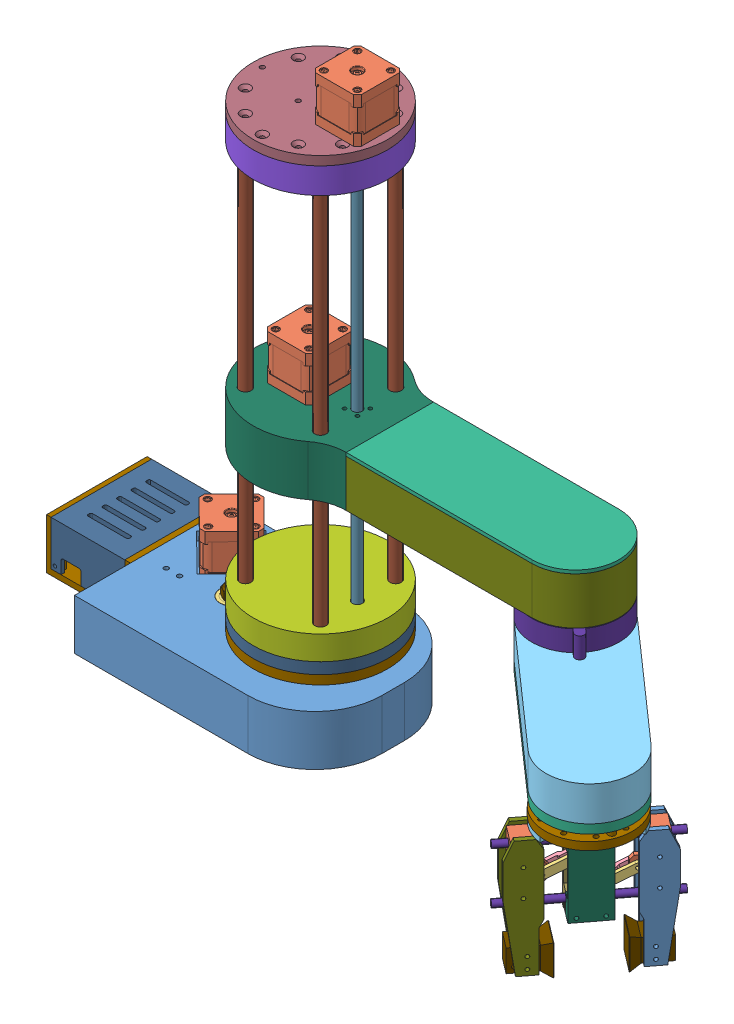
SolidWorks assembly SCARA Robot, configuration SCARA Robot. Lengths in mm. (continued)
Mates (geometry in assembly coordinates): (continued)
- Concentric43: concentric aligned: cylinder of Smooth Rod D10mm L400mm-2 through (76.0876 425 33.5876) axis (0 -1 0) radius 5; cylinder of Z-axis Mount Platform-1 through (76.0876 211.1984 33.5876) axis (0 -1 0) radius 5.25
- Concentric44: concentric anti-aligned: cylinder of Z-axis Mount Platform-1 through (-17.501 182.6984 -25.5) axis (1 0 0) radius 2.55; cylinder of Arm 1-1 through (309.501 182.6984 -25.5) axis (-1 0 0) radius 2.55
- Coincident31: coincident anti-aligned: plane of Z-axis Mount Platform-1 through (104.5 166.1984 0) normal (1 0 0); plane of Arm 1-1 through (104.5 176.1984 -39) normal (-1 0 0)
- Concentric451: concentric aligned: cylinder of Arm 1-1 through (180.5 182.1984 0) axis (0 -1 0) radius 11; cylinder of Ball Bearing 608 - 8x22x7mm-5 through (180.5 175.3984 0) axis (0 -1 0) radius 8.25
- Coincident321: coincident anti-aligned: plane of Arm 1-1 through (180.5 175.1984 0) normal (0 1 0); plane of Ball Bearing 608 - 8x22x7mm-5 through (180.5 175.1984 0) normal (0 -1 0)
- Coincident33: coincident anti-aligned: plane of Arm 1-1 through (180.5 173.1984 0) normal (0 -1 0); plane of Ball Bearing 608 - 8x22x7mm-6 through (180.5 173.1984 0) normal (0 1 0)
- Concentric46: concentric anti-aligned: cylinder of Arm 1-1 through (180.5 173.1984 0) axis (0 -1 0) radius 11; cylinder of Ball Bearing 608 - 8x22x7mm-6 through (180.5 166.1984 0) axis (0 1 0) radius 11
- Coincident34: coincident anti-aligned: plane of J2 Coupler-1 through (270.5 154.1984 0) normal (0 1 0); plane of Thrust Bearing 35x52x12mm-1 through (270.5 154.1984 0) normal (0 -1 0)
- Concentric47: concentric anti-aligned: cylinder of J2 Coupler-1 through (270.5 154.1984 0) axis (0 1 0) radius 26.5; cylinder of Thrust Bearing 35x52x12mm-1 through (270.5 166.1984 0) axis (0 -1 0) radius 26
- Concentric48: concentric anti-aligned: cylinder of Arm 1-1 through (270.5 169.1984 0) axis (0 1 0) radius 21; cylinder of Ball Bearing 30x42x7mm-1 through (270.5 176.1984 0) axis (0 -1 0) radius 21
- Coincident35: coincident anti-aligned: plane of Arm 1-1 through (270.5 169.1984 0) normal (0 1 0); plane of Ball Bearing 30x42x7mm-1 through (270.5 169.1984 0) normal (0 -1 0)
- Concentric49: concentric anti-aligned: cylinder of Arm 1-1 through (270.5 166.1984 0) axis (0 1 0) radius 17.5; cylinder of J2 Coupler-1 through (270.5 171.1984 0) axis (0 -1 0) radius 15
- Coincident36: coincident anti-aligned: plane of Arm 1-1 through (270.5 166.1984 0) normal (0 -1 0); plane of Thrust Bearing 35x52x12mm-1 through (270.5 166.1984 0) normal (0 1 0)
- Concentric50: concentric anti-aligned: cylinder of Ball Bearing 608 - 8x22x7mm-5 through (180.5 175.1984 0) axis (0 1 0) radius 4; cylinder of GT2 Pulley - 23 - 80 teeth-1 through (180.5 202.1984 0) axis (0 -1 0) radius 4
- Concentric51: concentric aligned: cylinder of J2 Coupler-1 through (270.5 147.1984 0) axis (0 1 0) radius 6.25; cylinder of GT2 Pulley - 92 teeth - J2-1 through (270.5 172.1984 0) axis (0 1 0) radius 6.25
- Coincident38: coincident anti-aligned: plane of GT2 Pulley - 92 teeth - J2-1 through (270.5 188.1984 0) normal (0 -1 0); plane of Thrust Bearing 35x52x12mm-2 through (270.5 188.1984 0) normal (0 1 0)
- Concentric52: concentric anti-aligned: cylinder of GT2 Pulley - 92 teeth - J2-1 through (270.5 172.1984 0) axis (0 1 0) radius 15; cylinder of Thrust Bearing 35x52x12mm-2 through (270.5 179.9984 0) axis (0 -1 0) radius 17.5
- Coincident39: coincident anti-aligned: plane of Arm 1-1 through (270.5 176.1984 0) normal (0 1 0); plane of Thrust Bearing 35x52x12mm-2 through (270.5 176.1984 0) normal (0 -1 0)
- Concentric53: concentric anti-aligned: cylinder of Z-axis Mount Platform-1 through (-17.501 200.6984 -25.5) axis (1 0 0) radius 2.55; cylinder of Arm 1-1 through (309.501 200.6984 -25.5) axis (-1 0 0) radius 2.55
- Concentric54: concentric aligned: cylinder of Z-axis Mount Platform-1 through (32.5 166.1984 0) axis (0 1 0) radius 12.5; cylinder of Stepper NEMA 17 -  20mm shaft-3 through (32.5 189.1984 0) axis (0 1 0) radius 2.5
- Concentric55: concentric anti-aligned: cylinder of Z-axis Mount Platform-1 through (17 166.1984 15.5) axis (0 1 0) radius 1.6; cylinder of Stepper NEMA 17 -  20mm shaft-3 through (17 215.1984 15.5) axis (0 -1 0) radius 1.5
- Coincident40: coincident anti-aligned: plane of Z-axis Mount Platform-1 through (42.5 211.1984 0) normal (0 1 0); plane of Stepper NEMA 17 -  20mm shaft-3 through (12 211.1984 0) normal (0 -1 0)
- Concentric56: concentric anti-aligned: cylinder of Stepper NEMA 17 -  20mm shaft-3 through (32.5 189.1984 0) axis (0 1 0) radius 2.5; cylinder of GT2 Pulley - Parametric-2 through (32.5 207.9984 0) axis (0 -1 0) radius 7.3122
- Coincident41: coincident aligned: plane of GT2 Pulley - 23 - 80 teeth-1 through (180.5 193.9984 0) normal (0 1 0); plane of GT2 Pulley - Parametric-2 through (32.5 193.9984 0) normal (0 1 0)
- Coincident42: coincident anti-aligned: plane of GT2 Pulley - 23 - 80 teeth-1 through (180.5 183.3984 0) normal (0 -1 0); plane of M8 Washer-3 through (180.5 183.3984 0) normal (0 1 0)
- Concentric57: concentric aligned: cylinder of GT2 Pulley - 23 - 80 teeth-1 through (180.5 202.1984 0) axis (0 -1 0) radius 4; cylinder of M8 Washer-3 through (180.5 183.3984 0) axis (0 -1 0) radius 7
- Coincident43: coincident anti-aligned: plane of Ball Bearing 608 - 8x22x7mm-5 through (180.5 182.1984 0) normal (0 1 0); plane of M8 Washer-3 through (180.5 182.1984 0) normal (0 -1 0)
- Concentric58: concentric anti-aligned: cylinder of Z-axis Mount Platform-1 through (8.9124 166.1984 33.5876) axis (0 1 0) radius 9.5; cylinder of Linear Bearing 10x19x29mm-3 through (8.9124 205.1984 33.5876) axis (0 -1 0) radius 9.5
- Coincident44: coincident anti-aligned: plane of Z-axis Mount Platform-1 through (104.4919 205.1984 81) normal (0 -1 0); plane of Linear Bearing 10x19x29mm-3 through (8.9124 205.1984 33.5876) normal (0 1 0)
- Coincident45: coincident anti-aligned: plane of Z-axis Mount Platform-1 through (104.4919 205.1984 81) normal (0 -1 0); plane of Linear Bearing 10x19x29mm-6 through (76.0876 205.1984 33.5876) normal (0 1 0)
- Concentric59: concentric anti-aligned: cylinder of Z-axis Mount Platform-1 through (76.0876 166.1984 33.5876) axis (0 1 0) radius 9.5; cylinder of Linear Bearing 10x19x29mm-6 through (76.0876 205.1984 33.5876) axis (0 -1 0) radius 5
- Concentric60: concentric anti-aligned: cylinder of Z-axis Mount Platform-1 through (76.0876 166.1984 -33.5876) axis (0 1 0) radius 9.5; cylinder of Linear Bearing 10x19x29mm-2 through (76.0876 205.1984 -33.5876) axis (0 -1 0) radius 9.5
- Coincident46: coincident anti-aligned: plane of Z-axis Mount Platform-1 through (104.4919 205.1984 81) normal (0 -1 0); plane of Linear Bearing 10x19x29mm-2 through (76.0876 205.1984 -33.5876) normal (0 1 0)
- Concentric61: concentric anti-aligned: cylinder of Z-axis Mount Platform-1 through (8.9124 166.1984 -33.5876) axis (0 1 0) radius 9.5; cylinder of Linear Bearing 10x19x29mm-1 through (8.9124 205.1984 -33.5876) axis (0 -1 0) radius 9.5
- Coincident47: coincident anti-aligned: plane of Z-axis Mount Platform-1 through (104.4919 205.1984 81) normal (0 -1 0); plane of Linear Bearing 10x19x29mm-1 through (8.9124 205.1984 -33.5876) normal (0 1 0)
- Parallel3: parallel aligned: plane of Base-1 through (-107.5 10 70) normal (0 0 1); plane of Arm 1-1 through (104.5 176.1984 39) normal (0 0 1)
- Concentric62: concentric aligned: cylinder of J2 Coupler-1 through (270.5 165.6984 0) axis (0 -1 0) radius 39; cylinder of Arm 2-1 through (270.5 147.1984 0) axis (0 -1 0) radius 17
- Coincident49: coincident anti-aligned: plane of J2 Coupler-1 through (270.5 147.1984 0) normal (0 -1 0); plane of Arm 2-1 through (270.5 147.1984 0) normal (0 1 0)
- Concentric63: concentric anti-aligned: cylinder of J2 Coupler-1 through (280.4501 147.1984 29.6236) axis (0 1 0) radius 2.05; cylinder of Arm 2-1 through (280.4501 147.1984 29.6236) axis (0 -1 0) radius 2.05
- Concentric64: concentric anti-aligned: cylinder of Arm 2-1 through (270.5 141.1984 0) axis (0 1 0) radius 39; cylinder of Arm 2 Cover-1 through (270.5 116.1984 0) axis (0 -1 0) radius 39
- Coincident50: coincident anti-aligned: plane of Arm 2-1 through (270.5 116.1984 0) normal (0 -1 0); plane of Arm 2 Cover-1 through (270.5 116.1984 0) normal (0 1 0)
- Concentric65: concentric anti-aligned: cylinder of Arm 2-1 through (378.46 141.1984 95.2924) axis (0 1 0) radius 39; cylinder of Arm 2 Cover-1 through (378.46 116.1984 95.2924) axis (0 -1 0) radius 39
- Concentric66: concentric anti-aligned: cylinder of Arm 1-1 through (220.888 166.1984 5) axis (0 1 0) radius 1.6; cylinder of Micro switch-1 through (220.888 166.1984 5) axis (0 -1 0) radius 1.5
- Concentric67: concentric anti-aligned: cylinder of Arm 1-1 through (212.5 166.1984 9.46) axis (0 1 0) radius 1.6; cylinder of Micro switch-1 through (212.5 166.1984 9.46) axis (0 -1 0) radius 1.5
- Coincident51: coincident anti-aligned: plane of Arm 1-1 through (270.5 166.1984 0) normal (0 -1 0); plane of Micro switch-1 through (217.6469 166.1984 9.5547) normal (0 1 0)
- Concentric68: concentric anti-aligned: cylinder of Arm 2 Cover-1 through (266.0017 108.1984 -3.9705) axis (0 1 0) radius 12.5; cylinder of NEMA 17 Stepper L24mm - 20mm shaft-1 through (266.0017 130.1984 -3.9705) axis (0 -1 0) radius 2.5
- Concentric69: concentric aligned: cylinder of Arm 2 Cover-1 through (267.3652 108.1984 17.9073) axis (0 1 0) radius 1.6; cylinder of NEMA 17 Stepper L24mm - 20mm shaft-1 through (267.3652 103.8984 17.9073) axis (0 1 0) radius 1.5
- Coincident52: coincident anti-aligned: plane of Arm 2 Cover-1 through (270.5 108.1984 0) normal (0 -1 0); plane of NEMA 17 Stepper L24mm - 20mm shaft-1 through (266.0017 108.1984 -3.9705) normal (0 1 0)
- Concentric701: concentric aligned: cylinder of Arm 2 Cover-1 through (372.8371 109.1984 90.3293) axis (0 1 0) radius 21; cylinder of Ball Bearing 30x42x7mm-2 through (372.8371 109.1984 90.3293) axis (0 1 0) radius 21
- Coincident53: coincident anti-aligned: plane of Arm 2 Cover-1 through (372.8371 109.1984 90.3293) normal (0 1 0); plane of Ball Bearing 30x42x7mm-2 through (372.8371 109.1984 90.3293) normal (0 -1 0)
- Concentric71: concentric anti-aligned: cylinder of Ball Bearing 30x42x7mm-2 through (372.8371 109.1984 90.3293) axis (0 1 0) radius 15; cylinder of Thrust Bearing 35x52x12mm-3 through (372.8371 119.9984 90.3293) axis (0 -1 0) radius 17.5
- Coincident54: coincident anti-aligned: plane of Arm 2 Cover-1 through (270.5 116.1984 0) normal (0 1 0); plane of Thrust Bearing 35x52x12mm-3 through (372.8371 116.1984 90.3293) normal (0 -1 0)
- Concentric73: concentric aligned: cylinder of Ball Bearing 30x42x7mm-2 through (372.8371 109.1984 90.3293) axis (0 1 0) radius 15; cylinder of Thrust Bearing 35x52x12mm-4 through (372.8371 96.1984 90.3293) axis (0 1 0) radius 17.5
- Coincident55: coincident anti-aligned: plane of Arm 2 Cover-1 through (270.5 108.1984 0) normal (0 -1 0); plane of Thrust Bearing 35x52x12mm-4 through (372.8371 108.1984 90.3293) normal (0 1 0)
- Concentric74: concentric anti-aligned: cylinder of J3 Coupler-1 through (372.8371 107.6984 90.3293) axis (0 -1 0) radius 26.5; cylinder of Thrust Bearing 35x52x12mm-4 through (372.8371 96.1984 90.3293) axis (0 1 0) radius 26
- Coincident56: coincident anti-aligned: plane of J3 Coupler-1 through (372.8371 96.1984 90.3293) normal (0 1 0); plane of Thrust Bearing 35x52x12mm-4 through (372.8371 96.1984 90.3293) normal (0 -1 0)
- Concentric75: concentric anti-aligned: cylinder of Thrust Bearing 35x52x12mm-3 through (372.8371 128.1984 90.3293) axis (0 -1 0) radius 17.5; cylinder of GT2 Pulley - 90 teeth - J3-1 through (372.8371 113.1984 90.3293) axis (0 1 0) radius 15
- Coincident57: coincident anti-aligned: plane of Thrust Bearing 35x52x12mm-3 through (372.8371 128.1984 90.3293) normal (0 1 0); plane of GT2 Pulley - 90 teeth - J3-1 through (372.8371 128.1984 90.3293) normal (0 -1 0)
- Concentric76: concentric anti-aligned: cylinder of NEMA 17 Stepper L24mm - 20mm shaft-1 through (266.0017 130.1984 -3.9705) axis (0 -1 0) radius 2.5; cylinder of GT2 Pulley - Parametric-3 through (266.0017 119.3984 -3.9705) axis (0 1 0) radius 7.3122
- Coincident58: coincident aligned: plane of GT2 Pulley - 90 teeth - J3-1 through (372.8371 126.3984 90.3293) normal (0 1 0); plane of GT2 Pulley - Parametric-3 through (266.0017 126.3984 -3.9705) normal (0 1 0)
- Concentric77: concentric aligned: cylinder of J3 Coupler-1 through (369.2 90.1984 100.7106) axis (0 1 0) radius 1.8; cylinder of GT2 Pulley - 90 teeth - J3-1 through (369.2 113.1984 100.7106) axis (0 1 0) radius 1.8
- Concentric78: concentric aligned: cylinder of J2 Coupler-1 through (259.7183 147.1984 -2.1806) axis (0 1 0) radius 1.8; cylinder of GT2 Pulley - 92 teeth - J2-1 through (259.7183 172.1984 -2.1806) axis (0 1 0) radius 1.8
- Coincident59: coincident anti-aligned: plane of Base-1 through (0 10 0) normal (0 1 0); plane of Micro switch-3 through (-8.7411 10 2.5547) normal (0 -1 0)
- Concentric79: concentric aligned: cylinder of Base-1 through (-5.5 10 -2) axis (0 -1 0) radius 1.6; cylinder of Micro switch-3 through (-5.5 16 -2) axis (0 -1 0) radius 1.5
- Concentric80: concentric aligned: cylinder of Base-1 through (-13.888 10 2.46) axis (0 -1 0) radius 1.6; cylinder of Micro switch-3 through (-13.888 16 2.46) axis (0 -1 0) radius 1.5
- Concentric81: concentric anti-aligned: cylinder of Arm 2 Cover-1 through (339.1646 108.1984 67.2769) axis (0 1 0) radius 1.6; cylinder of Micro switch-4 through (339.1646 108.1984 67.2769) axis (0 -1 0) radius 1.5
- Concentric82: concentric anti-aligned: cylinder of Arm 2 Cover-1 through (329.9245 108.1984 65.0698) axis (0 1 0) radius 1.6; cylinder of Micro switch-4 through (329.9245 108.1984 65.0698) axis (0 -1 0) radius 1.5
- Coincident60: coincident anti-aligned: plane of Arm 2 Cover-1 through (270.5 108.1984 0) normal (0 -1 0); plane of Micro switch-4 through (333.7206 108.1984 68.5469) normal (0 1 0)
- Concentric83: concentric anti-aligned: cylinder of Z-axis Mount Platform-1 through (75.5 207.1984 0) axis (0 -1 0) radius 5.1; cylinder of Lead Screw Nut 8mm-1 through (75.5 191.6984 0) axis (0 1 0) radius 5.1
- Concentric84: concentric anti-aligned: cylinder of Z-axis Mount Platform-1 through (81.25 211.1984 5.75) axis (0 -1 0) radius 1.6; cylinder of Lead Screw Nut 8mm-1 through (81.25 191.6974 5.75) axis (0 1 0) radius 1.5
- Coincident61: coincident anti-aligned: plane of Z-axis Mount Platform-1 through (104.4919 205.1984 81) normal (0 -1 0); plane of Lead Screw Nut 8mm-1 through (75.5 205.1984 0) normal (0 1 0)
- Coincident322: coincident anti-aligned: plane of J3 Coupler-1 through (372.8371 90.1984 90.3293) normal (0 -1 0); plane of Gripper Mechanism-1/Gripper to J3 connector-1 through (372.8371 90.1984 90.3293) normal (0 1 0)
- Concentric702: concentric anti-aligned: cylinder of J3 Coupler-1 through (400.587 90.1984 71.1197) axis (0 1 0) radius 2.05; cylinder of Gripper Mechanism-1/Gripper to J3 connector-1 through (400.587 90.1984 71.1197) axis (0 -1 0) radius 2.1
- Concentric703: concentric anti-aligned: cylinder of J3 Coupler-1 through (383.9961 90.1984 58.4775) axis (0 1 0) radius 2.05; cylinder of Gripper Mechanism-1/Gripper to J3 connector-1 through (383.9961 90.1984 58.4775) axis (0 -1 0) radius 2.1
- Coincident323: coincident anti-aligned: plane of Arm 1-1 through (270.5 208.1984 0) normal (0 1 0); plane of Arm 1 Cover-1 through (270.5 208.1984 0) normal (0 -1 0)
- Coincident324: coincident anti-aligned: plane of Z-axis Mount Platform-1 through (104.5 166.1984 0) normal (1 0 0); plane of Arm 1 Cover-1 through (104.5 208.1984 39) normal (-1 0 0)
- Coincident325: coincident aligned: plane of Arm 1-1 through (104.5 176.1984 39) normal (0 0 1); plane of Arm 1 Cover-1 through (270.5 208.1984 39) normal (0 0 1)
- Concentric704: concentric aligned: cylinder of Z-axis Top Plate-1 through (9.75 414.5 60) axis (0 0 -1) radius 1.6; cylinder of Micro switch-5 through (9.75 414.5 6) axis (0 0 -1) radius 1.5
- Concentric705: concentric aligned: cylinder of Z-axis Top Plate-1 through (19.25 414.5 60) axis (0 0 -1) radius 1.6; cylinder of Micro switch-5 through (19.25 414.5 6) axis (0 0 -1) radius 1.5
- Coincident326: coincident anti-aligned: plane of Z-axis Top Plate-1 through (4.5 407 0) normal (0 0 1); plane of Micro switch-5 through (14.25 412 0) normal (0 0 -1)
- Concentric706: concentric aligned: cylinder of Z-axis Top Plate-1 through (42.5 433 0) axis (0 -1 0) radius 60; cylinder of Top cover-1 through (42.5 404.5 0) axis (0 -1 0) radius 60
- Concentric707: concentric anti-aligned: cylinder of Z-axis Top Plate-1 through (42.5 425 52) axis (0 1 0) radius 2.05; cylinder of Top cover-1 through (42.5 425 52) axis (0 -1 0) radius 2.1
- Coincident327: coincident anti-aligned: plane of Z-axis Top Plate-1 through (42.5 425 0) normal (0 -1 0); plane of Top cover-1 through (42.5 425 0) normal (0 1 0)
- Concentric708: concentric anti-aligned: cylinder of Z-axis Bottom Plate-2 through (42.5 41 0) axis (0 -1 0) radius 60; cylinder of Base cover-1 through (42.5 60 0) axis (0 1 0) radius 60
- Concentric709: concentric aligned: cylinder of Lead Screw D8mm L380mm-1 through (75.5 413 0) axis (0 -1 0) radius 4; cylinder of Base cover-1 through (75.5 62.5 0) axis (0 -1 0) radius 4.5
- Coincident328: coincident anti-aligned: plane of Z-axis Bottom Plate-2 through (42.5 41 0) normal (0 1 0); plane of Base cover-1 through (42.5 41 0) normal (0 -1 0)
- Concentric710: concentric aligned: cylinder of Base-1 through (107.501 -13 -50) axis (-1 0 0) radius 2.05; cylinder of Arduino UNO case p1-1 through (-107.5 -13 -50) axis (-1 0 0) radius 2.1
- Coincident329: coincident anti-aligned: plane of Base-1 through (-107.5 10 70) normal (-1 0 0); plane of Arduino UNO case p1-1 through (-107.5 -32.5 20) normal (1 0 0)
- Concentric711: concentric aligned: cylinder of Base-1 through (107.501 -13 0) axis (-1 0 0) radius 2.05; cylinder of Arduino UNO case p1-1 through (-107.5 -13 0) axis (-1 0 0) radius 2.1
- Coincident331: coincident aligned: plane of Arduino UNO case p2-1 through (-145.5 8 20) normal (0 0 1); plane of Arduino UNO case p1-1 through (-145 -32.5 20) normal (0 0 1)
- Coincident332: coincident aligned: plane of Arduino UNO case p1-1 through (-145 10 20) normal (0 1 0); plane of Arduino UNO case p2-1 through (-178.5 10 20) normal (0 1 0)
- Coincident333: coincident anti-aligned: plane of Arduino UNO case p1-1 through (-112.5 -32.5 20) normal (-1 0 0); plane of Arduino UNO case p2-1 through (-112.5 6 20) normal (1 0 0)
- Concentric712: concentric aligned: cylinder of GT2 Pulley - Parametric-1 through (-69.2568 -12.3 -32.2954) axis (0 -1 0) radius 7.3122; cylinder of GT2 Belt 200mm-1 through (-69.2568 -19.3 -32.2954) axis (0 -1 0) radius 6.35
- Concentric713: concentric anti-aligned: cylinder of GT2 Pulley - 22 - 80 teeth-2 through (-36.5 -27.5 0) axis (0 1 0) radius 4; cylinder of GT2 Belt 200mm-1 through (-36.5 -19.3 0) axis (0 -1 0) radius 25.5
- Coincident334: coincident anti-aligned: plane of GT2 Pulley - Parametric-1 through (-69.2568 -19.3 -32.2954) normal (0 -1 0); plane of GT2 Belt 200mm-1 through (-69.2568 -19.3 -32.2954) normal (0 1 0)
- Concentric714: concentric aligned: cylinder of GT2 Pulley - 22 - 80 teeth-2 through (-36.5 -8.7 0) axis (0 -1 0) radius 7.9488; cylinder of GT2 Belt 300mm 2-1 through (-36.5 -11.2 0) axis (0 -1 0) radius 7
- Concentric716: concentric anti-aligned: cylinder of Thrust Bearing - 40x60x13-3 through (42.5 -3.8 0) axis (0 1 0) radius 30; cylinder of GT2 Belt 300mm 2-1 through (42.5 -11.2 0) axis (0 -1 0) radius 35
- Coincident335: coincident anti-aligned: plane of GT2 Pulley - 110 teeth - J1-2 through (42.5 -11.2 0) normal (0 -1 0); plane of GT2 Belt 300mm 2-1 through (-36.5 -11.2 0) normal (0 1 0)
- Concentric717: concentric aligned: cylinder of GT2 Pulley - 23 - 80 teeth-1 through (180.5 202.1984 0) axis (0 -1 0) radius 4; cylinder of GT2 Belt 400mm-1 through (180.5 200.9984 0) axis (0 -1 0) radius 25.5
- Concentric718: concentric aligned: cylinder of GT2 Pulley - Parametric-2 through (32.5 207.9984 0) axis (0 -1 0) radius 7.3122; cylinder of GT2 Belt 400mm-1 through (32.5 200.9984 0) axis (0 -1 0) radius 7.15
- Coincident336: coincident anti-aligned: plane of GT2 Pulley - Parametric-2 through (32.5 200.9984 0) normal (0 -1 0); plane of GT2 Belt 400mm-1 through (32.5 200.9984 0) normal (0 1 0)
- Concentric719: concentric anti-aligned: cylinder of GT2 Pulley - 23 - 80 teeth-1 through (180.5 191.5984 0) axis (0 1 0) radius 8.2671; cylinder of GT2 Belt 300mm-1 through (180.5 191.3984 0) axis (0 -1 0) radius 7.3
- Concentric720: concentric aligned: cylinder of GT2 Pulley - 92 teeth - J2-1 through (270.5 192.5984 0) axis (0 -1 0) radius 30.2305; cylinder of GT2 Belt 300mm-1 through (270.5 191.3984 0) axis (0 -1 0) radius 30.1
- Coincident337: coincident anti-aligned: plane of GT2 Pulley - 92 teeth - J2-1 through (270.5 191.3984 0) normal (0 -1 0); plane of GT2 Belt 300mm-1 through (180.5 191.3984 0) normal (0 1 0)
- Concentric721: concentric anti-aligned: cylinder of GT2 Pulley - 90 teeth - J3-1 through (372.8371 113.1984 90.3293) axis (0 1 0) radius 6.25; cylinder of GT2 Belt 400mm 2-1 through (372.8371 132.3984 90.3293) axis (0 -1 0) radius 28.65
- Concentric722: concentric anti-aligned: cylinder of GT2 Pulley - Parametric-3 through (266.0017 119.3984 -3.9705) axis (0 1 0) radius 7.3122; cylinder of GT2 Belt 400mm 2-1 through (266.0017 132.3984 -3.9705) axis (0 -1 0) radius 6.35
- Coincident338: coincident anti-aligned: plane of GT2 Pulley - 90 teeth - J3-1 through (372.8371 126.3984 90.3293) normal (0 1 0); plane of GT2 Belt 400mm 2-1 through (266.0017 126.3984 -3.9705) normal (0 -1 0)
- Concentric723: concentric aligned: cylinder of GT2 Pulley - 110 teeth - J1-2 through (42.5 3 0) axis (0 -1 0) radius 17.5; cylinder of Ball Bearing 35x47x7mm-1 through (42.5 7 0) axis (0 -1 0) radius 23.5
- Coincident339: coincident anti-aligned: plane of Base-1 through (42.5 7 0) normal (0 -1 0); plane of Ball Bearing 35x47x7mm-1 through (42.5 7 0) normal (0 1 0)
- Concentric724: concentric aligned: cylinder of GT2 Pulley - 22 - 80 teeth-2 through (-36.5 -27.5 0) axis (0 1 0) radius 4; cylinder of M8 45mm - Bolts-1 through (-36.5 -27.5 0) axis (0 1 0) radius 4
- Coincident340: coincident anti-aligned: plane of GT2 Pulley - 22 - 80 teeth-2 through (-36.5 -27.5 0) normal (0 -1 0); plane of M8 45mm - Bolts-1 through (-32.6456 -27.5 6.4402) normal (0 1 0)
- Concentric725: concentric anti-aligned: cylinder of M8 45mm - Bolts-1 through (-36.5 -27.5 0) axis (0 1 0) radius 4; cylinder of M8 Lock nut-1 through (-36.5 6 0) axis (0 -1 0) radius 4
- Coincident341: coincident anti-aligned: plane of Ball Bearing 608 - 8x22x7mm-2 through (-36.5 10 0) normal (0 1 0); plane of M8 Lock nut-1 through (-23.5191 10 -0.7051) normal (0 -1 0)
- Concentric727: concentric aligned: cylinder of GT2 Pulley - 23 - 80 teeth-1 through (180.5 202.1984 0) axis (0 -1 0) radius 4; cylinder of M8 45mm - Bolts-3 through (180.5 202.1984 0) axis (0 -1 0) radius 4
- Coincident342: coincident anti-aligned: plane of GT2 Pulley - 23 - 80 teeth-1 through (180.5 202.1984 0) normal (0 1 0); plane of M8 45mm - Bolts-3 through (173.0708 202.1984 -1.0681) normal (0 -1 0)
- Concentric728: concentric anti-aligned: cylinder of M8 45mm - Bolts-3 through (180.5 202.1984 0) axis (0 -1 0) radius 4; cylinder of M8 Lock nut-3 through (180.5 170.1984 0) axis (0 1 0) radius 4
- Coincident343: coincident anti-aligned: plane of Ball Bearing 608 - 8x22x7mm-6 through (180.5 166.1984 0) normal (0 -1 0); plane of M8 Lock nut-3 through (192.0993 166.1984 -5.87) normal (0 1 0)
- Concentric730: concentric aligned: cylinder of J1 coupler-1 through (42.5 31 -12.5) axis (0 1 0) radius 1.8; cylinder of M4 60mm - Bolts-1 through (42.5 31 -12.5) axis (0 1 0) radius 2
- Coincident345: coincident aligned: plane of J1 coupler-1 through (42.5 31 0) normal (0 1 0); plane of M4 60mm - Bolts-1 through (40.5876 31 -11.9146) normal (0 1 0)
- Concentric731: concentric aligned: cylinder of J1 coupler-1 through (30 31 0) axis (0 1 0) radius 1.8; cylinder of M4 60mm - Bolts-2 through (30 31 0) axis (0 1 0) radius 2
- Coincident346: coincident aligned: plane of J1 coupler-1 through (42.5 31 0) normal (0 1 0); plane of M4 60mm - Bolts-2 through (30 31 -2) normal (0 1 0)
- Concentric732: concentric aligned: cylinder of J1 coupler-1 through (55 31 0) axis (0 1 0) radius 1.8; cylinder of M4 60mm - Bolts-3 through (55 31 0) axis (0 1 0) radius 2
- Coincident347: coincident aligned: plane of J1 coupler-1 through (42.5 31 0) normal (0 1 0); plane of M4 60mm - Bolts-3 through (55 31 -2) normal (0 1 0)
- Concentric733: concentric aligned: cylinder of J1 coupler-1 through (42.5 31 12.5) axis (0 1 0) radius 1.8; cylinder of M4 60mm - Bolts-4 through (42.5 31 12.5) axis (0 1 0) radius 2
- Coincident348: coincident aligned: plane of J1 coupler-1 through (42.5 31 0) normal (0 1 0); plane of M4 60mm - Bolts-4 through (42.5 31 10.5) normal (0 1 0)
- Concentric734: concentric anti-aligned: cylinder of J2 Coupler-1 through (259.7183 147.1984 -2.1806) axis (0 1 0) radius 1.8; cylinder of M4 50mm - Bolts-1 through (259.7183 147.1984 -2.1806) axis (0 -1 0) radius 2
- Coincident349: coincident aligned: plane of J2 Coupler-1 through (270.5 147.1984 0) normal (0 -1 0); plane of M4 50mm - Bolts-1 through (259.7183 147.1984 -0.1806) normal (0 -1 0)
- Concentric735: concentric anti-aligned: cylinder of J2 Coupler-1 through (268.3194 147.1984 10.7817) axis (0 1 0) radius 1.8; cylinder of M4 50mm - Bolts-2 through (268.3194 147.1984 10.7817) axis (0 -1 0) radius 2
- Coincident350: coincident aligned: plane of J2 Coupler-1 through (270.5 147.1984 0) normal (0 -1 0); plane of M4 50mm - Bolts-2 through (268.3194 147.1984 12.7817) normal (0 -1 0)
- Concentric736: concentric anti-aligned: cylinder of J2 Coupler-1 through (281.2817 147.1984 2.1806) axis (0 1 0) radius 1.8; cylinder of M4 50mm - Bolts-3 through (281.2817 147.1984 2.1806) axis (0 -1 0) radius 2
- Coincident351: coincident aligned: plane of J2 Coupler-1 through (270.5 147.1984 0) normal (0 -1 0); plane of M4 50mm - Bolts-3 through (281.2817 147.1984 4.1806) normal (0 -1 0)
- Concentric737: concentric anti-aligned: cylinder of J2 Coupler-1 through (272.6806 147.1984 -10.7817) axis (0 1 0) radius 1.8; cylinder of M4 50mm - Bolts-4 through (272.6806 147.1984 -10.7817) axis (0 -1 0) radius 2
- Coincident352: coincident aligned: plane of J2 Coupler-1 through (270.5 147.1984 0) normal (0 -1 0); plane of M4 50mm - Bolts-4 through (272.6806 147.1984 -8.7817) normal (0 -1 0)
- Concentric738: concentric aligned: cylinder of M4 Lock nut-1 through (259.7183 190.5984 -2.1806) axis (0 -1 0) radius 2; cylinder of M4 50mm - Bolts-1 through (259.7183 147.1984 -2.1806) axis (0 -1 0) radius 2
- Coincident353: coincident anti-aligned: plane of GT2 Pulley - 92 teeth - J2-1 through (270.5 192.5984 0) normal (0 1 0); plane of M4 Lock nut-1 through (259.7183 192.5984 -6.222) normal (0 -1 0)
- Concentric739: concentric aligned: cylinder of M4 Lock nut-2 through (272.6806 190.5984 -10.7817) axis (0 -1 0) radius 2; cylinder of M4 50mm - Bolts-4 through (272.6806 147.1984 -10.7817) axis (0 -1 0) radius 2
- Coincident354: coincident aligned: plane of M4 Lock nut-1 through (259.7183 197.5984 -6.222) normal (0 1 0); plane of M4 Lock nut-2 through (272.6806 197.5984 -14.8232) normal (0 1 0)
- Concentric740: concentric aligned: cylinder of M4 Lock nut-3 through (281.2817 190.5984 2.1806) axis (0 -1 0) radius 2; cylinder of M4 50mm - Bolts-3 through (281.2817 147.1984 2.1806) axis (0 -1 0) radius 2
- Concentric741: concentric aligned: cylinder of M4 Lock nut-4 through (268.3194 190.5984 10.7817) axis (0 -1 0) radius 2; cylinder of M4 50mm - Bolts-2 through (268.3194 147.1984 10.7817) axis (0 -1 0) radius 2
- Coincident355: coincident aligned: plane of M4 Lock nut-1 through (259.7183 197.5984 -6.222) normal (0 1 0); plane of M4 Lock nut-4 through (268.3194 197.5984 6.7403) normal (0 1 0)
- Coincident356: coincident aligned: plane of M4 Lock nut-1 through (259.7183 197.5984 -6.222) normal (0 1 0); plane of M4 Lock nut-3 through (281.2817 197.5984 -1.8609) normal (0 1 0)
- Coincident357: coincident anti-aligned: plane of GT2 Pulley - 110 teeth - J1-2 through (42.5 -19.4 0) normal (0 -1 0); plane of M4 Lock nut-5 through (44.7104 -19.4 9.1166) normal (0 1 0)
- Concentric742: concentric aligned: cylinder of M4 60mm - Bolts-4 through (42.5 31 12.5) axis (0 1 0) radius 2; cylinder of M4 Lock nut-5 through (42.5 -17.4 12.5) axis (0 1 0) radius 2
- Coincident358: coincident anti-aligned: plane of GT2 Pulley - 110 teeth - J1-2 through (42.5 -19.4 0) normal (0 -1 0); plane of M4 Lock nut-7 through (57.2104 -19.4 -3.3834) normal (0 1 0)
- Concentric743: concentric aligned: cylinder of M4 60mm - Bolts-3 through (55 31 0) axis (0 1 0) radius 2; cylinder of M4 Lock nut-7 through (55 -17.4 0) axis (0 1 0) radius 2
- Coincident359: coincident anti-aligned: plane of GT2 Pulley - 110 teeth - J1-2 through (42.5 -19.4 0) normal (0 -1 0); plane of M4 Lock nut-6 through (44.7104 -19.4 -15.8834) normal (0 1 0)
- Concentric744: concentric aligned: cylinder of M4 60mm - Bolts-1 through (42.5 31 -12.5) axis (0 1 0) radius 2; cylinder of M4 Lock nut-6 through (42.5 -17.4 -12.5) axis (0 1 0) radius 2
- Coincident360: coincident anti-aligned: plane of GT2 Pulley - 110 teeth - J1-2 through (42.5 -19.4 0) normal (0 -1 0); plane of M4 Lock nut-8 through (32.2104 -19.4 -3.3834) normal (0 1 0)
- Concentric745: concentric aligned: cylinder of M4 60mm - Bolts-2 through (30 31 0) axis (0 1 0) radius 2; cylinder of M4 Lock nut-8 through (30 -17.4 0) axis (0 1 0) radius 2
